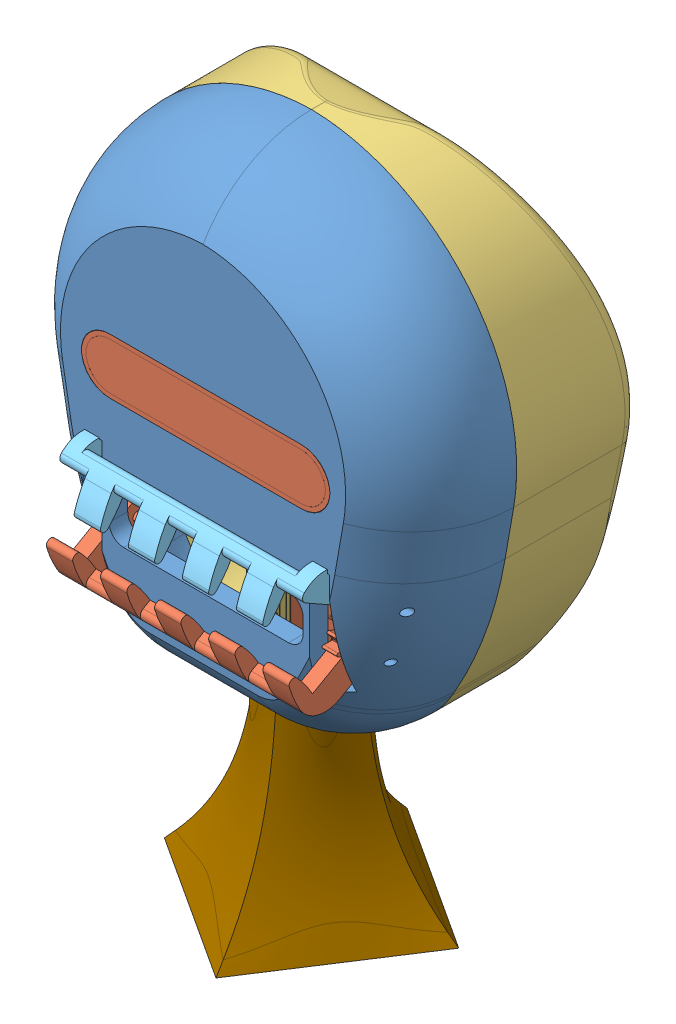
SolidWorks assembly assembly head of jaloul, configuration Défaut. Lengths in mm.
Overall size (153.86 218.57 97.38).
54 component instances, 42 part files, 20 mates.
Components (placement in the parent):
- head of jaloul-1: head of jaloul [Défaut] at (-2.8889 8.1989 56.9742) size (153.86 167.94 40.08)
- RealSense_D435-1: RealSense_D435 [Default] at (-2 5.7058 43.2445) size (90.75 24.75 24.23)
- ras jaloul men teli-1: ras jaloul men teli [Défaut] at (-4.3071 -4.0651 25.143) size (140.75 169.26 46.26)
- raspberry-pi-5-sbc-simple.step-1: raspberry-pi-5-sbc-simple.step [Défaut] at (-2.8895 30.0633 18.143) size (90.56 58 19.2)
  - CSI_DSI-1.step-1: CSI_DSI-1.step [Défaut] at (-70.5 -36 11.75) size (3 15.5 4.1)
    - CSI_DSI_connector.step-1: CSI_DSI_connector.step [Défaut] at origin size (3 15.5 4.1)
  - CSI_DSI-2.step-1: CSI_DSI-2.step [Défaut] at (-70.5 -36 11.75) size (3 15.5 4.1)
    - CSI_DSI_connector.step-1: CSI_DSI_connector.step [Défaut] at (6.2 0 0) size (3 15.5 4.1)
  - pcba-components.step-1: pcba-components.step [Défaut] at (-70.5 -36 11.75) size (64.89 40.96 3.37)
    - pcba-components Geometry.step-1: pcba-components Geometry.step [Défaut] at origin size (62.02 39.27 3.37)
    - chips.step-1: chips.step [Défaut] at origin size (13.6 15 1)
  - poe.step-1: poe.step [Défaut] at (-70.5 -36 11.75) size (5.08 5.08 8.29)
    - poe Geometry.step-1: poe Geometry.step [Défaut] at origin size (5.08 5.08 1)
    - poe-pins.step-1: poe-pins.step [Défaut] at origin size (3.44 3.44 7.29)
  - usb-2-bank.step-1: usb-2-bank.step [Défaut] at (-0.7443 20 0.8) x (1 0 0) z (0 -1 0) size (17.07 15.5 13.76)
    - usb-2-bank Geometry.step-1: usb-2-bank Geometry.step [Défaut] at origin size (16.67 15.5 13.76)
    - usb2-port.step-1: usb2-port.step [Défaut] at origin size (4.42 5.12 12.5)
    - usb2-port.step-2: usb2-port.step [Défaut] at (0 -8.5 0) size (4.42 5.12 12.5)
  - usb-3-bank.step-1: usb-3-bank.step [Défaut] at (-0.5443 2.1 0.8) x (1 0 0) z (0 -1 0) size (17.07 15.5 13.76)
    - usb-3-bank Geometry.step-1: usb-3-bank Geometry.step [Défaut] at origin size (16.67 15.5 13.76)
    - usb3-port.step-1: usb3-port.step [Défaut] at origin size (4.42 5.12 12.5)
    - usb3-port.step-2: usb3-port.step [Défaut] at (0 -8.5 0) size (4.42 5.12 12.5)
  - connector.step-1: connector.step [Défaut] at (-70.5 -36 11.75) size (3 6 3.5)
  - ethernet.step-1: ethernet.step [Défaut] at (0 -35.55 0.8) x (1 0 0) z (0 -1 0) size (23.65 17.25 16)
  - gpio.step-1: gpio.step [Défaut] at (-70.53 -36.28 11.75) size (50.5 5 8.29)
  - hdmi-micro.step-1: hdmi-micro.step [Défaut] at (-0.3 0 0.8) x (1 0 0) z (0 -1 0) size (6.5 2.9 7.7)
  - hdmi-micro.step-2: hdmi-micro.step [Défaut] at (-13.8 0 0.8) x (1 0 0) z (0 -1 0) size (6.5 2.9 7.7)
  - IR.step-1: IR.step [Défaut] at (-70.5 -36 11.75) size (1.73 3.15 3.26)
  - mounting-holes.step-1: mounting-holes.step [Défaut] at (-70.5 -36 11.75) size (64 54.91 0.02)
  - pcb.step-1: pcb.step [Défaut] at (-70.5 -36 11.75) size (85 56 1.6)
  - pcie.step-1: pcie.step [Défaut] at (-70.5 -36 11.75) size (3 10.5 4.1)
  - pmic.step-1: pmic.step [Défaut] at (-70.5 -36 11.75) size (6 6 0.5)
  - pwr-connector.step-1: pwr-connector.step [Défaut] at (-70.5 -36 11.75) size (4 3 4.4)
  - rp1.step-1: rp1.step [Défaut] at (-70.5 -36 11.75) size (12 12 0.5)
  - sd-card.step-1: sd-card.step [Défaut] at (-70.5 -36 11.75) size (1.75 11.01 0.01) (hidden)
  - switch.step-1: switch.step [Défaut] at (-70.5 -36 11.75) size (3 4.75 1.77)
  - uart.step-1: uart.step [Défaut] at (-70.5 -36 11.75) size (5.25 3.25 4.4)
  - usb-c.step-1: usb-c.step [Défaut] at (-70.5 -36 11.75) size (9 7.5 3.2)
- support head-1: support head [Défaut] at (-2.8895 -82.9367 30.143) x (0.544466 0 -0.838783) z (0 -1 0) size (62.95 62.95 55.38)
- M90S_ali.step-1: M90S_ali.step [Défaut] at (23.3 -47.0367 54.243) x (0 -1 0) z (1 0 0) size (32.3 12.4 32.5)
  - axe.step-1: axe.step [Défaut] at origin size (4.9 4.9 14.2)
  - base001.step-1: base001.step [Défaut] at origin size (32.3 12.2 28.5)
  - etiquette.step-1: etiquette.step [Défaut] at origin size (20 0.2 10)
  - Tube.step-1: Tube.step [Défaut] at (5.4 0 -13.3) x (0 0 -1) z (1 0 0) size (1.2 1.2 3)
  - Cylindre.step-1: Cylindre.step [Défaut] at (5.4 0 -13.3) x (0 0 -1) z (1 0 0) size (0.4 0.4 4)
  - Tube001.step-1: Tube001.step [Défaut] at (5.4 -1.2 -13.3) x (0 0 -1) z (1 0 0) size (1.2 1.2 3)
  - Tube002.step-1: Tube002.step [Défaut] at (5.4 1.2 -13.3) x (0 0 -1) z (1 0 0) size (1.2 1.2 3)
  - etiquette001.step-1: etiquette001.step [Défaut] at (-10.8 0 0) x (-1 0 0) z (0 0 1) size (20 0.2 10)
  - Cylindre001.step-1: Cylindre001.step [Défaut] at (5.4 1.2 -13.3) x (0 0 -1) z (1 0 0) size (0.4 0.4 4)
  - Cylindre002.step-1: Cylindre002.step [Défaut] at (5.4 -1.2 -13.3) x (0 0 -1) z (1 0 0) size (0.4 0.4 4)
- dents du jaloul-1: dents du jaloul [Défaut] at (-1.85 -55.3304 58.7391) x (-1 0 0) z (0 0.870081 0.492909) size (83 33.18 25.45)
- MG90S_arm01.step-1: MG90S_arm01.step [Défaut] at (39.3 -47.0367 54.243) x (-1 0 0) z (0 0.870081 0.492909) size (4.8 21.4 6.8)
- dent jaloul partie supérieur-1: dent jaloul partie supérieur [Défaut] at (-1.85 5.574 3.1017) size (83 33.18 25.45)
- Symétriedents du jaloul-4: Symétriedents du jaloul [Défaut] at (-1.85 -21.043 58.7391) x (-1 0 0) z (0 0.870081 -0.492909) size (83 32.99 25.26)
Mates (geometry in assembly coordinates):
- Coïncidente1: coincident aligned: plane of head of jaloul-1 through (-2.8895 28.2077 67.2445) normal (0 0 1); plane of RealSense_D435-1 through (-2 5.7058 67.2445) normal (0 0 1)
- Distance1: distance = 60 mm: line of RealSense_D435-1 through (31.1879 -6.5684 59.9405) axis (-1 0 0); line of head of jaloul-1 through (-21.2343 -66.5612 60.8695) axis (1 0 0)
- Distance4: distance = 2 mm: axis of RealSense_D435-1 through (-2 -4.1684 53.8219) axis (0 -1 0)
- Coïncidente6: coincident anti-aligned: plane of head of jaloul-1 through (-2.8895 79.0866 30.143) normal (0 0 -1); plane of ras jaloul men teli-1 through (-4.1483 7.7202 30.143) normal (0 0 1)
- Coïncidente7: coincident aligned: line of head of jaloul-1 through (-20.696 -87.9367 30.143) axis (1 0 0); line of ras jaloul men teli-1 through (-21.7726 -87.9367 30.143) axis (1 0 0)
- Coïncidente8: coincident aligned: circle of head of jaloul-1; circle of ras jaloul men teli-1
- Coïncidente9: coincident anti-aligned: plane of ras jaloul men teli-1 through (-4.3071 -4.0651 18.143) normal (0 0 1); plane of raspberry-pi-5-sbc-simple.step-1/pcb.step-1 through (-73.3895 -5.9367 18.143) normal (0 0 -1)
- Distance5: distance = 85 mm anti-aligned: plane of raspberry-pi-5-sbc-simple.step-1/pcb.step-1 through (39.6105 2.0633 19.743) normal (0 -1 0); plane of ras jaloul men teli-1 through (-4.3071 -82.9367 18.143) normal (0 1 0)
- Largeur1: width aligned: plane of raspberry-pi-5-sbc-simple.step-1/pcb.step-1 through (-45.3895 2.0633 19.743) normal (-1 0 0); plane of raspberry-pi-5-sbc-simple.step-1/pcb.step-1 through (39.6105 58.0633 19.743) normal (1 0 0); plane of ras jaloul men teli-1 through (-65.0631 -14.778 18.143) normal (0.984808 0.173648 0); plane of ras jaloul men teli-1 through (59.1986 -15.2628 18.143) normal (-0.984808 0.173648 0)
- Coaxiale1: concentric aligned: cylinder of head of jaloul-1 through (-2.8895 -87.9638 30.143) axis (0 1 0) radius 15; cylinder of support head-1 through (-2.8895 -122.9367 30.143) axis (0 1 0) radius 15
- Coïncidente11: coincident aligned: plane of ras jaloul men teli-1 through (-4.3071 -82.9367 18.143) normal (0 1 0); plane of support head-1 through (-2.8895 -82.9367 30.143) normal (0 1 0)
- Distance9: distance = 30 mm anti-aligned: plane of ras jaloul men teli-1 through (-4.3071 -4.0651 18.143) normal (0 0 1); plane of M90S_ali.step-1/base001.step-1 through (17.8374 -41.5867 48.143) normal (0 0 -1)
- Distance6: distance = 30 mm anti-aligned: plane of M90S_ali.step-1/base001.step-1 through (23.3 -52.9367 60.343) normal (0 -1 0); plane of support head-1 through (-2.8895 -82.9367 30.143) normal (0 1 0)
- Distance7: distance = 5 mm anti-aligned: plane of M90S_ali.step-1/base001.step-1 through (5 -41.5867 54.243) normal (-1 0 0)
- Coaxiale2: concentric aligned: cylinder of M90S_ali.step-1/base001.step-1 through (27.8 -47.0367 54.243) axis (-1 0 0) radius 6; cylinder of dents du jaloul-1 through (39.65 -47.0367 54.243) axis (-1 0 0) radius 1.5
- Coaxiale4: concentric anti-aligned: cylinder of M90S_ali.step-1/base001.step-1 through (27.8 -47.0367 54.243) axis (-1 0 0) radius 6; cylinder of MG90S_arm01.step-1 through (39.3 -47.0367 54.243) axis (1 0 0) radius 3.4
- Coïncidente19: coincident anti-aligned: plane of M90S_ali.step-1/axe.step-1 through (37.5 -47.0367 54.243) normal (1 0 0); plane of MG90S_arm01.step-1 through (37.5 -46.4649 55.538) normal (-1 0 0)
- Distance8: distance = 2 mm aligned: plane of MG90S_arm01.step-1 through (36.65 -50.5186 60.3892) normal (-1 0 0); plane of dents du jaloul-1 through (34.65 -51.5587 72.369) normal (-1 0 0)
- Coïncidente21: coincident aligned: plane of dents du jaloul-1 through (39.65 -54.0232 76.7194) normal (1 0 0); plane of dent jaloul partie supérieur-1 through (39.65 20.574 13.1017) normal (1 0 0)
- Largeur2: width anti-aligned: plane of dents du jaloul-1 through (-1.85 -46.6296 63.6681) normal (0 0.870081 0.492909); plane of MG90S_arm01.step-1 through (-1.85 -55.3304 58.7391) normal (0 -0.870081 -0.492909); plane of dents du jaloul-1 through (38.8 -44.2364 56.1713) normal (0 0.823614 0.567151); plane of MG90S_arm01.step-1 through (38.8 -50.1303 52.8323) normal (0 -0.909873 -0.414887)
